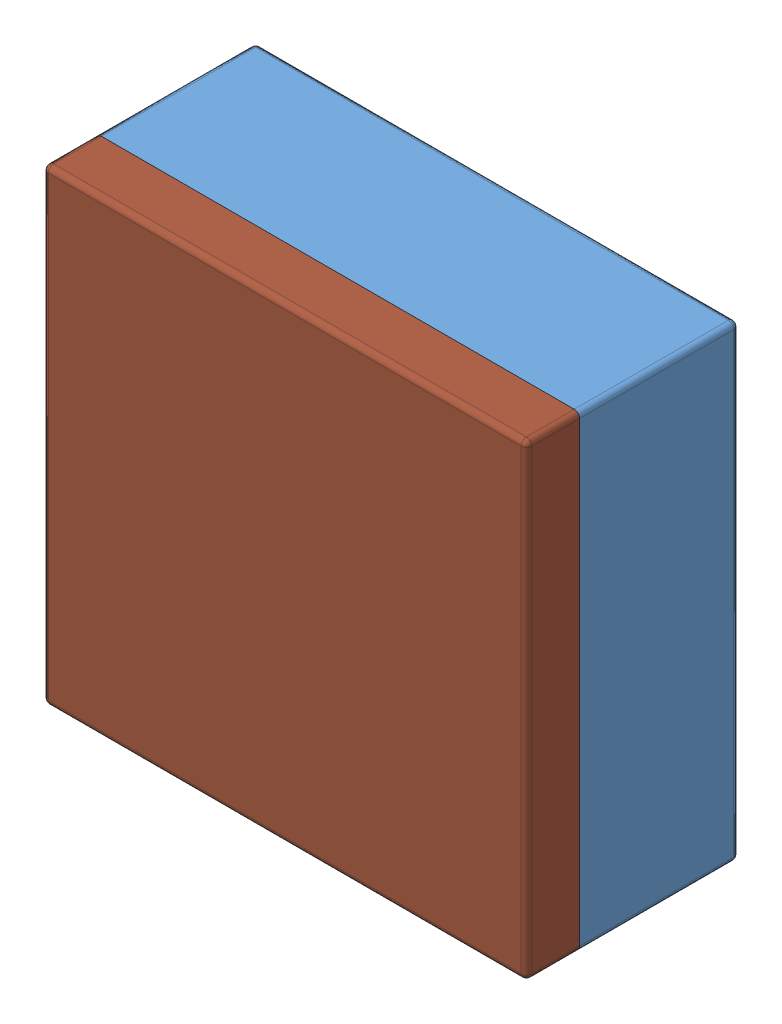
SolidWorks assembly Assem1, configuration Default. Lengths in mm. (continued)
Components (placement in the parent): (continued)
- Assem147-1: Assem147 [Default] at (118.0608 24.9039 43.2392) size (91 88 30) (continued)
  - Main Controller.step-1: Main Controller.step [Default] at (-5.5498 -47.3965 22.6108) x (0 1 0) z (0 0 1) size (83.62 86.87 19.5) (continued)
    - J8.step-1: J8.step [Default] at origin size (3.8 20 9.2) (continued)
      - Conn_JST_B7B-EH-A_LF_SN_eec.step-1: Conn_JST_B7B-EH-A_LF_SN_eec.step [Default] at (52.405 60.267 0) x (0 -1 0) z (0 0 1) size (20 3.8 9.2) (continued)
        - Notch.step-1: Notch.step [Default] at (-10.3528 -1.902 -5.8229) x (1 0 0) z (0 1 0) size (0.19 0.26 0)
    - J7.step-1: J7.step [Default] at origin size (5.75 12.4 10.4)
      - Conn_JST_B4B-XH-A_LF_SN_eec.step-1: Conn_JST_B4B-XH-A_LF_SN_eec.step [Default] at (29.828 73.64 0) x (0 1 0) z (0 0 1) size (12.4 5.75 10.4)
        - 1-45.step-1: 1-45.step [Default] x (1 0 0) z (0 -1 0) size (8.14 10.3 0.9)
        - 2-46.step-1: 2-46.step [Default] x (1 0 0) z (0 -1 0) size (12.4 7 5.75)
        - Pin1_Triangle.step-1: Pin1_Triangle.step [Default] at (-3.7456 -2.776 -1.3492) x (1 0 0) z (0 -1 0) size (0.89 0.61 0.02)
        - JST.step-1: JST.step [Default] at (6.1995 1.4972 0.8858) x (0 1 0) z (1 0 0) size (1.59 0.67 0.01)
    - J6.step-1: J6.step [Default] at origin size (12.4 5.75 10.4)
      - Conn_JST_B4B-XH-A_LF_SN_eec.step-1: Conn_JST_B4B-XH-A_LF_SN_eec.step [Default] at (46.034 121.048 0) x (-1 0 0) z (0 0 1) size (12.4 5.75 10.4)
        - 1-45.step-1: 1-45.step [Default] x (1 0 0) z (0 -1 0) size (8.14 10.3 0.9)
        - 2-46.step-1: 2-46.step [Default] x (1 0 0) z (0 -1 0) size (12.4 7 5.75)
        - Pin1_Triangle.step-1: Pin1_Triangle.step [Default] at (-3.7456 -2.776 -1.3492) x (1 0 0) z (0 -1 0) size (0.89 0.61 0.02)
        - JST.step-1: JST.step [Default] at (6.1995 1.4972 0.8858) x (0 1 0) z (1 0 0) size (1.59 0.67 0.01)
    - J5.step-1: J5.step [Default] at origin size (9.62 5 8.9)
      - 690368170672.step-1: 690368170672.step [Default] at (40.4959 71.009 3.35) x (1 0 0) z (0 1 0) size (9.62 8.9 5)
        - 690368170672-50.step-1: 690368170672-50.step [Default] at origin size (9.62 5 5)
        - Pin_2.step-1: Pin_2.step [Default] at (-1.905 0 1) size (0.55 7.9 5)
        - Pin.step-1: Pin.step [Default] at (1.905 0 1) x (-1 0 0) z (0 0 1) size (0.55 7.9 5)
        - Pin.step-2: Pin.step [Default] at (-0.635 0 1) x (-1 0 0) z (0 0 1) size (0.55 7.9 5)
        - Pin_2.step-2: Pin_2.step [Default] at (0.635 0 1) size (0.55 7.9 5)
        - Pin_2.step-3: Pin_2.step [Default] at (3.175 0 1) size (0.55 7.9 5)
        - Pin.step-3: Pin.step [Default] at (-3.175 0 1) x (-1 0 0) z (0 0 1) size (0.55 7.9 5)
    - J2.step-1: J2.step [Default] at origin size (12.4 5.75 10.4)
      - Conn_JST_B4B-XH-A_LF_SN_eec.step-1: Conn_JST_B4B-XH-A_LF_SN_eec.step [Default] at (42.311 62.086 0) x (-1 0 0) z (0 0 1) size (12.4 5.75 10.4)
        - 1-45.step-1: 1-45.step [Default] x (1 0 0) z (0 -1 0) size (8.14 10.3 0.9)
        - 2-46.step-1: 2-46.step [Default] x (1 0 0) z (0 -1 0) size (12.4 7 5.75)
        - Pin1_Triangle.step-1: Pin1_Triangle.step [Default] at (-3.7456 -2.776 -1.3492) x (1 0 0) z (0 -1 0) size (0.89 0.61 0.02)
        - JST.step-1: JST.step [Default] at (6.1995 1.4972 0.8858) x (0 1 0) z (1 0 0) size (1.59 0.67 0.01)
    - J1.step-1: J1.step [Default] at origin size (12.4 5.75 10.4)
      - Conn_JST_B4B-XH-A_LF_SN_eec.step-1: Conn_JST_B4B-XH-A_LF_SN_eec.step [Default] at (91.2943 121.048 0) x (-1 0 0) z (0 0 1) size (12.4 5.75 10.4)
        - 1-45.step-1: 1-45.step [Default] x (1 0 0) z (0 -1 0) size (8.14 10.3 0.9)
        - 2-46.step-1: 2-46.step [Default] x (1 0 0) z (0 -1 0) size (12.4 7 5.75)
        - Pin1_Triangle.step-1: Pin1_Triangle.step [Default] at (-3.7456 -2.776 -1.3492) x (1 0 0) z (0 -1 0) size (0.89 0.61 0.02)
        - JST.step-1: JST.step [Default] at (6.1995 1.4972 0.8858) x (0 1 0) z (1 0 0) size (1.59 0.67 0.01)
    - IC1.step-1: IC1.step [Default] at origin size (7 2.7 2)
      - 6352349152.step-1: 6352349152.step [Default] at (61.595 88.138 0) x (-1 0 0) z (0 0 1) size (7 2.7 2)
        - Body-51.step-1: Body-51.step [Default] at origin size (4.4 2.7 1.95)
        - PinsArrayLR-52.step-1: PinsArrayLR-52.step [Default] at origin size (7 1.67 1.12)
    - F1.step-1: F1.step [Default] at origin size (6.16 4.91 1.71)
      - 6352355232.step-1: 6352355232.step [Default] at (38.608 114.655 0) size (6.16 4.91 1.71)
        - term1.step-1: term1.step [Default] at (-2.275 -1.62 0) size (0.3 3.24 0.85)
        - term2.step-1: term2.step [Default] at (1.975 -1.62 0) size (0.3 3.24 0.85)
        - Body.step-1: Body.step [Default] at (-1.975 -1.5876 0.0085) size (3.82 3.4 1.7)
    - D1.step-1: D1.step [Default] at origin size (1.3 2.92 1.1)
      - 6357170608.step-1: 6357170608.step [Default] at (83.677 114.495 0.01) size (1.3 2.92 1.1)
        - Extruded-53.step-1: Extruded-53.step [Default] at origin size (1.3 2.92 1.1)
    - C17.step-1: C17.step [Default] at origin size (2.2 1.45 1.45)
      - 6357171088.step-1: 6357171088.step [Default] at (45.378 84.709 0) size (0.5 1.45 1.45)
        - Extruded-54.step-1: Extruded-54.step [Default] at origin size (0.5 1.45 1.45)
      - 6357171088.step-2: 6357171088.step [Default] at (47.078 84.709 0) size (0.5 1.45 1.45)
        - Extruded-54.step-1: Extruded-54.step [Default] at origin size (0.5 1.45 1.45)
      - 6357170848.step-1: 6357170848.step [Default] at (46.228 84.709 0) size (1.2 1.45 1.45)
        - Extruded-55.step-1: Extruded-55.step [Default] at origin size (1.2 1.45 1.45)
    - C16.step-1: C16.step [Default] at origin size (2.2 1.45 1.45)
      - 6357171088.step-1: 6357171088.step [Default] at (45.378 87.376 0) size (0.5 1.45 1.45)
        - Extruded-54.step-1: Extruded-54.step [Default] at origin size (0.5 1.45 1.45)
      - 6357171088.step-2: 6357171088.step [Default] at (47.078 87.376 0) size (0.5 1.45 1.45)
        - Extruded-54.step-1: Extruded-54.step [Default] at origin size (0.5 1.45 1.45)
      - 6357170848.step-1: 6357170848.step [Default] at (46.228 87.376 0) size (1.2 1.45 1.45)
        - Extruded-55.step-1: Extruded-55.step [Default] at origin size (1.2 1.45 1.45)
    - C15.step-1: C15.step [Default] at origin size (0.6 0.3 0.34)
      - Cap_Murata_GRM0335C1HR30BA01D_eec.step-1: Cap_Murata_GRM0335C1HR30BA01D_eec.step [Default] at (47.4367 95.504 0) x (-1 0 0) z (0 0 1) size (0.6 0.3 0.34)
        - terminals.step-1: terminals.step [Default] at origin size (0.6 0.3 0.33)
        - body-56.step-1: body-56.step [Default] at origin size (0.3 0.3 0.33)
        - logo.step-1: logo.step [Default] at (-0.2332 0.5956 0.33) size (0.25 0.06 0.01)
    - C14.step-1: C14.step [Default] at origin size (2.2 1.45 1.45)
      - 6357171088.step-1: 6357171088.step [Default] at (45.378 89.789 0) size (0.5 1.45 1.45)
        - Extruded-54.step-1: Extruded-54.step [Default] at origin size (0.5 1.45 1.45)
      - 6357171088.step-2: 6357171088.step [Default] at (47.078 89.789 0) size (0.5 1.45 1.45)
        - Extruded-54.step-1: Extruded-54.step [Default] at origin size (0.5 1.45 1.45)
      - 6357170848.step-1: 6357170848.step [Default] at (46.228 89.789 0) size (1.2 1.45 1.45)
        - Extruded-55.step-1: Extruded-55.step [Default] at origin size (1.2 1.45 1.45)
    - C13.step-1: C13.step [Default] at origin size (1.25 2 1.4)
      - Cap_Murata_GRM21BC81C106KA73L_eec.step-1: Cap_Murata_GRM21BC81C106KA73L_eec.step [Default] at (49.276 115.145 0) x (0 -1 0) z (0 0 1) size (2 1.25 1.4)
        - 1-57.step-1: 1-57.step [Default] at origin size (2 1.25 1.4)
        - 2-58.step-1: 2-58.step [Default] at (0 0 0.01) size (1.98 1.23 1.38)
        - Murata_Logo_3.step-1: Murata_Logo_3.step [Default] at (-0.1814 -0.5957 1.2901) size (0.53 0.12 0.1)
    - C12.step-1: C12.step [Default] at origin size (0.6 0.3 0.34)
      - Cap_Murata_GRM0335C1HR30BA01D_eec.step-1: Cap_Murata_GRM0335C1HR30BA01D_eec.step [Default] at (45.0243 98.806 0) x (-1 0 0) z (0 0 1) size (0.6 0.3 0.34)
        - terminals.step-1: terminals.step [Default] at origin size (0.6 0.3 0.33)
        - body-56.step-1: body-56.step [Default] at origin size (0.3 0.3 0.33)
        - logo.step-1: logo.step [Default] at (-0.2332 0.5956 0.33) size (0.25 0.06 0.01)
    - C11.step-1: C11.step [Default] at origin size (3.2 1.6 0.88)
      - Cap_KEMET_C1206C472K4RACTU_eec.step-1: Cap_KEMET_C1206C472K4RACTU_eec.step [Default] at (38.1 92.8848 0) x (1 0 0) z (0 0 1) size (3.2 1.6 0.88)
      - Cap_KEMET_C1206C472K4RACTU_eec-59.step-1: Cap_KEMET_C1206C472K4RACTU_eec-59.step [Default] at (38.1 92.8848 0) x (1 0 0) z (0 0 1) size (2.2 1.5 0.78)
      - Cap_KEMET_C1206C472K4RACTU_eec-60.step-1: Cap_KEMET_C1206C472K4RACTU_eec-60.step [Default] at (38.1 92.8848 0) x (1 0 0) z (0 0 1) size (0.88 0.18 0)
    - C10.step-1: C10.step [Default] at origin size (0.6 0.3 0.34)
      - Cap_Murata_GRM0335C1HR30BA01D_eec.step-1: Cap_Murata_GRM0335C1HR30BA01D_eec.step [Default] at (45.0243 101.092 0) x (-1 0 0) z (0 0 1) size (0.6 0.3 0.34)
        - terminals.step-1: terminals.step [Default] at origin size (0.6 0.3 0.33)
        - body-56.step-1: body-56.step [Default] at origin size (0.3 0.3 0.33)
        - logo.step-1: logo.step [Default] at (-0.2332 0.5956 0.33) size (0.25 0.06 0.01)
    - C9.step-1: C9.step [Default] at origin size (2 1.25 1.4)
      - Cap_Murata_GRM21BC81C106KA73L_eec.step-1: Cap_Murata_GRM21BC81C106KA73L_eec.step [Default] at (46.421 105.41 0) x (-1 0 0) z (0 0 1) size (2 1.25 1.4)
        - 1-57.step-1: 1-57.step [Default] at origin size (2 1.25 1.4)
        - 2-58.step-1: 2-58.step [Default] at (0 0 0.01) size (1.98 1.23 1.38)
        - Murata_Logo_3.step-1: Murata_Logo_3.step [Default] at (-0.1814 -0.5957 1.2901) size (0.53 0.12 0.1)
    - C8.step-1: C8.step [Default] at origin size (2 1.25 1.4)
      - Cap_Murata_GRM21BC81C106KA73L_eec.step-1: Cap_Murata_GRM21BC81C106KA73L_eec.step [Default] at (37.5 95.4025 0) size (2 1.25 1.4)
        - 1-57.step-1: 1-57.step [Default] at origin size (2 1.25 1.4)
        - 2-58.step-1: 2-58.step [Default] at (0 0 0.01) size (1.98 1.23 1.38)
        - Murata_Logo_3.step-1: Murata_Logo_3.step [Default] at (-0.1814 -0.5957 1.2901) size (0.53 0.12 0.1)
    - C7.step-1: C7.step [Default] at origin size (0.6 0.3 0.34)
      - Cap_Murata_GRM0335C1HR30BA01D_eec.step-1: Cap_Murata_GRM0335C1HR30BA01D_eec.step [Default] at (45.0243 94.742 0) x (-1 0 0) z (0 0 1) size (0.6 0.3 0.34)
        - terminals.step-1: terminals.step [Default] at origin size (0.6 0.3 0.33)
        - body-56.step-1: body-56.step [Default] at origin size (0.3 0.3 0.33)
        - logo.step-1: logo.step [Default] at (-0.2332 0.5956 0.33) size (0.25 0.06 0.01)
    - C6.step-1: C6.step [Default] at origin size (0.6 0.3 0.34)
      - Cap_Murata_GRM0335C1HR30BA01D_eec.step-1: Cap_Murata_GRM0335C1HR30BA01D_eec.step [Default] at (45.0243 96.393 0) size (0.6 0.3 0.34)
        - terminals.step-1: terminals.step [Default] at origin size (0.6 0.3 0.33)
        - body-56.step-1: body-56.step [Default] at origin size (0.3 0.3 0.33)
        - logo.step-1: logo.step [Default] at (-0.2332 0.5956 0.33) size (0.25 0.06 0.01)
    - C5.step-1: C5.step [Default] at origin size (2.2 1.45 1.45)
      - 6357171088.step-1: 6357171088.step [Default] at (36.525 98.0953 0) size (0.5 1.45 1.45)
        - Extruded-54.step-1: Extruded-54.step [Default] at origin size (0.5 1.45 1.45)
      - 6357171088.step-2: 6357171088.step [Default] at (38.225 98.0953 0) size (0.5 1.45 1.45)
        - Extruded-54.step-1: Extruded-54.step [Default] at origin size (0.5 1.45 1.45)
      - 6357170848.step-1: 6357170848.step [Default] at (37.375 98.0953 0) size (1.2 1.45 1.45)
        - Extruded-55.step-1: Extruded-55.step [Default] at origin size (1.2 1.45 1.45)
    - 3-61.step-1: 3-61.step [Default] at origin size (1.65 3.25 0.7)
      - 6357168288.step-1: 6357168288.step [Default] at (75.946 110.595 0) size (1.65 0.5 0.7)
        - Extruded-62.step-1: Extruded-62.step [Default] at origin size (1.65 0.5 0.7)
      - 6357168288.step-2: 6357168288.step [Default] at (75.946 107.845 0) size (1.65 0.5 0.7)
        - Extruded-62.step-1: Extruded-62.step [Default] at origin size (1.65 0.5 0.7)
      - 6357168048.step-1: 6357168048.step [Default] at (75.946 109.22 0) size (1.65 2.25 0.7)
        - Extruded-63.step-1: Extruded-63.step [Default] at origin size (1.65 2.25 0.7)
    - 5.step-1: 5.step [Default] at origin size (1.65 3.25 0.7)
      - 6357168288.step-1: 6357168288.step [Default] at (75.946 105.134 0) size (1.65 0.5 0.7)
        - Extruded-62.step-1: Extruded-62.step [Default] at origin size (1.65 0.5 0.7)
      - 6357168288.step-2: 6357168288.step [Default] at (75.946 102.384 0) size (1.65 0.5 0.7)
        - Extruded-62.step-1: Extruded-62.step [Default] at origin size (1.65 0.5 0.7)
      - 6357168048.step-1: 6357168048.step [Default] at (75.946 103.759 0) size (1.65 2.25 0.7)
        - Extruded-63.step-1: Extruded-63.step [Default] at origin size (1.65 2.25 0.7)
    - 4.step-1: 4.step [Default] at origin size (1.05 0.55 0.4)
      - 6352350512.step-1: 6352350512.step [Default] at (79.5201 110.998 0) x (1 0 0) z (0 0 1) size (1.05 0.55 0.4)
        - Terminal-4.step-1: Terminal-4.step [Default] at (-0.525 -0.275 0) size (0.2 0.55 0.4)
          - Open_CASCADE_STEP_translator_6.8_9.2.1-64.step-1: Open_CASCADE_STEP_translator_6.8_9.2.1-64.step [Default] at origin size (0.2 0.55 0.4)
        - Terminal-4.step-2: Terminal-4.step [Default] at (0.525 0.275 0) x (-1 0 0) z (0 0 1) size (0.2 0.55 0.4)
          - Open_CASCADE_STEP_translator_6.8_9.2.1-64.step-1: Open_CASCADE_STEP_translator_6.8_9.2.1-64.step [Default] at origin size (0.2 0.55 0.4)
        - Mid_Body-65.step-1: Mid_Body-65.step [Default] at (-0.525 -0.275 0) size (0.97 0.55 0.32)
        - Mark-66.step-1: Mark-66.step [Default] at (-0.325 -0.275 0.36) size (0.65 0.55 0.04)
    - 3-1.step-1: 3-1.step [Default] at origin size (1.05 0.55 0.4)
      - 6352340032.step-1: 6352340032.step [Default] at (80.245 107.442 0) x (-1 0 0) z (0 0 1) size (1.05 0.55 0.4)
        - Terminal-5.step-1: Terminal-5.step [Default] at (-0.525 -0.275 0) size (0.2 0.55 0.4)
          - Open_CASCADE_STEP_translator_6.8_9.2.1-67.step-1: Open_CASCADE_STEP_translator_6.8_9.2.1-67.step [Default] at origin size (0.2 0.55 0.4)
        - Terminal-5.step-2: Terminal-5.step [Default] at (0.525 0.275 0) x (-1 0 0) z (0 0 1) size (0.2 0.55 0.4)
          - Open_CASCADE_STEP_translator_6.8_9.2.1-67.step-1: Open_CASCADE_STEP_translator_6.8_9.2.1-67.step [Default] at origin size (0.2 0.55 0.4)
        - Mid_Body-68.step-1: Mid_Body-68.step [Default] at (-0.525 -0.275 0) size (0.97 0.55 0.32)
        - Mark-69.step-1: Mark-69.step [Default] at (-0.325 -0.275 0.36) size (0.65 0.55 0.04)
    - 2-1.step-1: 2-1.step [Default] at origin size (1.05 0.55 0.4)
      - 6352350512.step-1: 6352350512.step [Default] at (75.596 99.314 0) x (1 0 0) z (0 0 1) size (1.05 0.55 0.4)
        - Terminal-4.step-1: Terminal-4.step [Default] at (-0.525 -0.275 0) size (0.2 0.55 0.4)
          - Open_CASCADE_STEP_translator_6.8_9.2.1-64.step-1: Open_CASCADE_STEP_translator_6.8_9.2.1-64.step [Default] at origin size (0.2 0.55 0.4)
        - Terminal-4.step-2: Terminal-4.step [Default] at (0.525 0.275 0) x (-1 0 0) z (0 0 1) size (0.2 0.55 0.4)
          - Open_CASCADE_STEP_translator_6.8_9.2.1-64.step-1: Open_CASCADE_STEP_translator_6.8_9.2.1-64.step [Default] at origin size (0.2 0.55 0.4)
        - Mid_Body-65.step-1: Mid_Body-65.step [Default] at (-0.525 -0.275 0) size (0.97 0.55 0.32)
        - Mark-66.step-1: Mark-66.step [Default] at (-0.325 -0.275 0.36) size (0.65 0.55 0.04)
    - 1-1.step-1: 1-1.step [Default] at origin size (1.05 0.55 0.4)
      - 6352350512.step-1: 6352350512.step [Default] at (75.596 97.155 0) x (1 0 0) z (0 0 1) size (1.05 0.55 0.4)
        - Terminal-4.step-1: Terminal-4.step [Default] at (-0.525 -0.275 0) size (0.2 0.55 0.4)
          - Open_CASCADE_STEP_translator_6.8_9.2.1-64.step-1: Open_CASCADE_STEP_translator_6.8_9.2.1-64.step [Default] at origin size (0.2 0.55 0.4)
        - Terminal-4.step-2: Terminal-4.step [Default] at (0.525 0.275 0) x (-1 0 0) z (0 0 1) size (0.2 0.55 0.4)
          - Open_CASCADE_STEP_translator_6.8_9.2.1-64.step-1: Open_CASCADE_STEP_translator_6.8_9.2.1-64.step [Default] at origin size (0.2 0.55 0.4)
        - Mid_Body-65.step-1: Mid_Body-65.step [Default] at (-0.525 -0.275 0) size (0.97 0.55 0.32)
        - Mark-66.step-1: Mark-66.step [Default] at (-0.325 -0.275 0.36) size (0.65 0.55 0.04)
    - SW1.step-1: SW1.step [Default] at origin size (6.4 5.1 2.05)
      - 6352340512.step-1: 6352340512.step [Default] at (30.9307 118.237 0) size (6.4 5.1 2.05)
    - R6.step-1: R6.step [Default] at origin size (0.55 1.05 0.4)
      - 6352352672.step-1: 6352352672.step [Default] at (52.07 97.3481 0) x (0 1 0) z (0 0 1) size (1.05 0.55 0.4)
        - Terminal-2.step-1: Terminal-2.step [Default] at (-0.525 -0.275 0) size (0.2 0.55 0.4)
          - Open_CASCADE_STEP_translator_6.8_9.2.1-31.step-1: Open_CASCADE_STEP_translator_6.8_9.2.1-31.step [Default] at origin size (0.2 0.55 0.4)
        - Terminal-2.step-2: Terminal-2.step [Default] at (0.525 0.275 0) x (-1 0 0) z (0 0 1) size (0.2 0.55 0.4)
          - Open_CASCADE_STEP_translator_6.8_9.2.1-31.step-1: Open_CASCADE_STEP_translator_6.8_9.2.1-31.step [Default] at origin size (0.2 0.55 0.4)
        - Mid_Body-32.step-1: Mid_Body-32.step [Default] at (-0.525 -0.275 0) size (0.97 0.55 0.32)
        - Mark-33.step-1: Mark-33.step [Default] at (-0.325 -0.275 0.36) size (0.65 0.55 0.04)
    - R1.step-1: R1.step [Default] at origin size (0.8 1.6 0.63)
      - Res_Panasonic_ERJ-3EKF12R0V_eec.step-1: Res_Panasonic_ERJ-3EKF12R0V_eec.step [Default] at (68.58 96.901 0) x (0 -1 0) z (0 0 1) size (1.6 0.8 0.63)
        - body-70.step-1: body-70.step [Default] at (0 0 0.5) x (1 0 0) z (0 0 -1) size (1.5 0.8 0.45)
        - pad.step-1: pad.step [Default] at (-0.6133 -0.4 0.55) x (1 0 0) z (0 1 0) size (0.3 0.55 0.8)
        - pad.step-2: pad.step [Default] at (0.6133 0.4 0.55) x (-1 0 0) z (0 -1 0) size (0.3 0.55 0.8)
        - top.step-1: top.step [Default] at (0 0 0.05) x (1 0 0) z (0 0 -1) size (1 0.8 0.05)
        - top.step-2: top.step [Default] at (0 0 0.55) x (1 0 0) z (0 0 -1) size (1 0.8 0.05)
        - Panasonic.step-1: Panasonic.step [Default] at (0.8789 -0.1125 0.55) size (0.9 0.17 0.15)
    - MD1.step-1: MD1.step [Default] at origin size (25.5 18.01 3.25)
      - UNK_Espressif_Systems_ESP32-WROOM-32E_4MB_eec.step-1: UNK_Espressif_Systems_ESP32-WROOM-32E_4MB_eec.step [Default] at (96.393 93.345 0) x (0 -1 0) z (0 0 1) size (18 25.5 3.25)
        - 1-71.step-1: 1-71.step [Default] at origin size (18 25.5 0.6)
        - 4-72.step-1: 4-72.step [Default] at origin size (15.81 5.41 0.1)
        - 5-73.step-1: 5-73.step [Default] at origin size (15.8 17.61 2.65)
        - 6.step-1: 6.step [Default] at origin size (18 25.5 0.46)
        - 3-74.step-1: 3-74.step [Default] at origin size (0.45 0.9 0.6)
        - 3-74.step-2: 3-74.step [Default] at (0 1.27 0) size (0.45 0.9 0.6)
        - 3-74.step-3: 3-74.step [Default] at (0 2.54 0) size (0.45 0.9 0.6)
        - 3-74.step-4: 3-74.step [Default] at (0 3.81 0) size (0.45 0.9 0.6)
        - 3-74.step-5: 3-74.step [Default] at (0 5.08 0) size (0.45 0.9 0.6)
        - 3-74.step-6: 3-74.step [Default] at (0 6.35 0) size (0.45 0.9 0.6)
        - 3-74.step-7: 3-74.step [Default] at (0 7.62 0) size (0.45 0.9 0.6)
        - 3-74.step-8: 3-74.step [Default] at (0 8.89 0) size (0.45 0.9 0.6)
        - 3-74.step-9: 3-74.step [Default] at (0 10.16 0) size (0.45 0.9 0.6)
        - 3-74.step-10: 3-74.step [Default] at (0 11.43 0) size (0.45 0.9 0.6)
        - 3-74.step-11: 3-74.step [Default] at (0 12.7 0) size (0.45 0.9 0.6)
        - 3-74.step-12: 3-74.step [Default] at (0 13.97 0) size (0.45 0.9 0.6)
        - 3-74.step-13: 3-74.step [Default] at (0 15.24 0) size (0.45 0.9 0.6)
        - 3-74.step-14: 3-74.step [Default] at (0 16.51 0) size (0.45 0.9 0.6)
        - 3_MIR.step-1: 3_MIR.step [Default] x (-1 0 0) z (0 0 -1) size (0.45 0.9 0.6)
        - 3_MIR.step-2: 3_MIR.step [Default] at (0 1.27 0) x (-1 0 0) z (0 0 -1) size (0.45 0.9 0.6)
        - 3_MIR.step-3: 3_MIR.step [Default] at (0 2.54 0) x (-1 0 0) z (0 0 -1) size (0.45 0.9 0.6)
        - 3_MIR.step-4: 3_MIR.step [Default] at (0 3.81 0) x (-1 0 0) z (0 0 -1) size (0.45 0.9 0.6)
        - 3_MIR.step-5: 3_MIR.step [Default] at (0 5.08 0) x (-1 0 0) z (0 0 -1) size (0.45 0.9 0.6)
        - 3_MIR.step-6: 3_MIR.step [Default] at (0 6.35 0) x (-1 0 0) z (0 0 -1) size (0.45 0.9 0.6)
        - 3_MIR.step-7: 3_MIR.step [Default] at (0 7.62 0) x (-1 0 0) z (0 0 -1) size (0.45 0.9 0.6)
        - 3_MIR.step-8: 3_MIR.step [Default] at (0 8.89 0) x (-1 0 0) z (0 0 -1) size (0.45 0.9 0.6)
        - 3_MIR.step-9: 3_MIR.step [Default] at (0 10.16 0) x (-1 0 0) z (0 0 -1) size (0.45 0.9 0.6)
        - 3_MIR.step-10: 3_MIR.step [Default] at (0 11.43 0) x (-1 0 0) z (0 0 -1) size (0.45 0.9 0.6)
        - 3_MIR.step-11: 3_MIR.step [Default] at (0 12.7 0) x (-1 0 0) z (0 0 -1) size (0.45 0.9 0.6)
        - 3_MIR.step-12: 3_MIR.step [Default] at (0 13.97 0) x (-1 0 0) z (0 0 -1) size (0.45 0.9 0.6)
        - 3_MIR.step-13: 3_MIR.step [Default] at (0 15.24 0) x (-1 0 0) z (0 0 -1) size (0.45 0.9 0.6)
        - 3_MIR.step-14: 3_MIR.step [Default] at (0 16.51 0) x (-1 0 0) z (0 0 -1) size (0.45 0.9 0.6)
        - 2-75.step-1: 2-75.step [Default] at origin size (0.9 0.45 0.6)
        - 2-75.step-2: 2-75.step [Default] at (1.27 0 0) size (0.9 0.45 0.6)
        - 2-75.step-3: 2-75.step [Default] at (2.54 0 0) size (0.9 0.45 0.6)
        - 2-75.step-4: 2-75.step [Default] at (3.81 0 0) size (0.9 0.45 0.6)
        - 2-75.step-5: 2-75.step [Default] at (5.08 0 0) size (0.9 0.45 0.6)
        - 2-75.step-6: 2-75.step [Default] at (6.35 0 0) size (0.9 0.45 0.6)
        - 2-75.step-7: 2-75.step [Default] at (7.62 0 0) size (0.9 0.45 0.6)
        - 2-75.step-8: 2-75.step [Default] at (8.89 0 0) size (0.9 0.45 0.6)
        - 2-75.step-9: 2-75.step [Default] at (10.16 0 0) size (0.9 0.45 0.6)
        - 2-75.step-10: 2-75.step [Default] at (11.43 0 0) size (0.9 0.45 0.6)
        - Espressif__Logo.step-1: Espressif__Logo.step [Default] at (-3.7229 6.4842 3.151) size (14.63 2.95 0.1)
        - 7.step-1: 7.step [Default] at origin size (3.7 3.7 0)
    - JP3.step-1: JP3.step [Default] at origin size (5.75 7.4 10.4)
      - Conn_JST_B2B-XH-A_LF_SN_eec.step-1: Conn_JST_B2B-XH-A_LF_SN_eec.step [Default] at (29.828 86.1245 0) x (0 1 0) z (0 0 1) size (7.4 5.75 10.4)
        - 1-43.step-1: 1-43.step [Default] at (0 0.025 0) x (-1 0 0) z (0 1 0) size (7.4 10.4 5.75)
          - 1-44.step-1: 1-44.step [Default] at origin size (3.14 10.2 0.64)
          - B2B-XH-A.step-1: B2B-XH-A.step [Default] at origin size (7.4 7 5.75)
          - JST_Logo_adjustable.step-1: JST_Logo_adjustable.step [Default] at (-1.7267 5.5034 2.841) size (0.85 2.3 0.01)
    - JP2.step-1: JP2.step [Default] at origin size (5.75 12.4 10.4)
      - Conn_JST_B4B-XH-A_LF_SN_eec.step-1: Conn_JST_B4B-XH-A_LF_SN_eec.step [Default] at (29.828 97.8636 0) x (0 1 0) z (0 0 1) size (12.4 5.75 10.4)
        - 1-45.step-1: 1-45.step [Default] x (1 0 0) z (0 -1 0) size (8.14 10.3 0.9)
        - 2-46.step-1: 2-46.step [Default] x (1 0 0) z (0 -1 0) size (12.4 7 5.75)
        - Pin1_Triangle.step-1: Pin1_Triangle.step [Default] at (-3.7456 -2.776 -1.3492) x (1 0 0) z (0 -1 0) size (0.89 0.61 0.02)
        - JST.step-1: JST.step [Default] at (6.1995 1.4972 0.8858) x (0 1 0) z (1 0 0) size (1.59 0.67 0.01)
    - JP1.step-1: JP1.step [Default] at origin size (5.75 7.4 10.4)
      - Conn_JST_B2B-XH-A_LF_SN_eec.step-1: Conn_JST_B2B-XH-A_LF_SN_eec.step [Default] at (29.828 109.7428 0) x (0 1 0) z (0 0 1) size (7.4 5.75 10.4)
        - 1-43.step-1: 1-43.step [Default] at (0 0.025 0) x (-1 0 0) z (0 1 0) size (7.4 10.4 5.75)
          - 1-44.step-1: 1-44.step [Default] at origin size (3.14 10.2 0.64)
          - B2B-XH-A.step-1: B2B-XH-A.step [Default] at origin size (7.4 7 5.75)
          - JST_Logo_adjustable.step-1: JST_Logo_adjustable.step [Default] at (-1.7267 5.5034 2.841) size (0.85 2.3 0.01)
    - C4.step-1: C4.step [Default] at origin size (0.6 0.3 0.34)
      - Cap_Murata_GRM0335C1HR30BA01D_eec.step-1: Cap_Murata_GRM0335C1HR30BA01D_eec.step [Default] at (47.4367 97.2217 0) x (-1 0 0) z (0 0 1) size (0.6 0.3 0.34)
        - terminals.step-1: terminals.step [Default] at origin size (0.6 0.3 0.33)
        - body-56.step-1: body-56.step [Default] at origin size (0.3 0.3 0.33)
        - logo.step-1: logo.step [Default] at (-0.2332 0.5956 0.33) size (0.25 0.06 0.01)
    - C3.step-1: C3.step [Default] at origin size (2 1.25 1.4)
      - Cap_Murata_GRM21BC81C106KA73L_eec.step-1: Cap_Murata_GRM21BC81C106KA73L_eec.step [Default] at (37.5 100.838 0) x (-1 0 0) z (0 0 1) size (2 1.25 1.4)
        - 1-57.step-1: 1-57.step [Default] at origin size (2 1.25 1.4)
        - 2-58.step-1: 2-58.step [Default] at (0 0 0.01) size (1.98 1.23 1.38)
        - Murata_Logo_3.step-1: Murata_Logo_3.step [Default] at (-0.1814 -0.5957 1.2901) size (0.53 0.12 0.1)
    - C2.step-1: C2.step [Default] at origin size (0.6 0.3 0.34)
      - Cap_Murata_GRM0335C1HR30BA01D_eec.step-1: Cap_Murata_GRM0335C1HR30BA01D_eec.step [Default] at (47.4367 98.806 0) x (-1 0 0) z (0 0 1) size (0.6 0.3 0.34)
        - terminals.step-1: terminals.step [Default] at origin size (0.6 0.3 0.33)
        - body-56.step-1: body-56.step [Default] at origin size (0.3 0.3 0.33)
        - logo.step-1: logo.step [Default] at (-0.2332 0.5956 0.33) size (0.25 0.06 0.01)
    - C1.step-1: C1.step [Default] at origin size (0.6 0.3 0.34)
      - Cap_Murata_GRM0335C1HR30BA01D_eec.step-1: Cap_Murata_GRM0335C1HR30BA01D_eec.step [Default] at (47.4367 100.965 0) x (-1 0 0) z (0 0 1) size (0.6 0.3 0.34)
        - terminals.step-1: terminals.step [Default] at origin size (0.6 0.3 0.33)
        - body-56.step-1: body-56.step [Default] at origin size (0.3 0.3 0.33)
        - logo.step-1: logo.step [Default] at (-0.2332 0.5956 0.33) size (0.25 0.06 0.01)
- 2nd top-1: 2nd top [Default] at (-16.29 1.2345 98.8925) x (0 1 0) z (0 0 -1) size (88 91 10)
Mates (geometry in assembly coordinates):
- Coincident1: coincident: line of Assem147-1/2nd below-1 through (-15.29 1.2345 88.8925) axis (1 0 0); line of 2nd top-1 through (73.71 1.2345 88.8925) axis (-1 0 0)
- Coincident2: coincident aligned: plane of Assem147-1/2nd below-1 through (74.71 1.2345 88.8925) normal (1 0 0); plane of 2nd top-1 through (74.71 1.2345 88.8925) normal (1 0 0)
